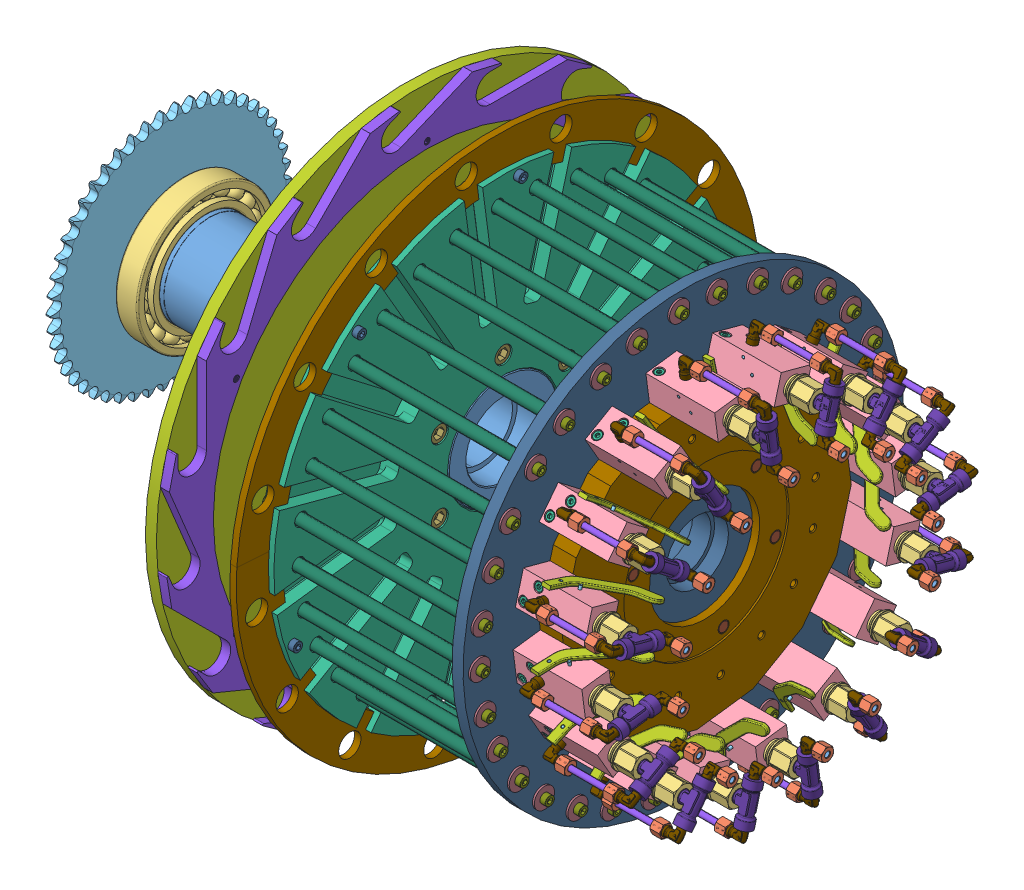
SolidWorks assembly assieme parte rotante, configuration Default. Lengths in mm. (continued)
Components (placement in the parent): (continued)
- AssiemeValvola-7: AssiemeValvola [Default] at (515.3257 -116.5064 518.4894) x (0 0.793353 -0.608761) z (0 -0.608761 -0.793353) size (90.26 138.63 38)
  - RaccordoT-1: RaccordoT [Default] at origin size (43 29.75 16.5)
  - Raccordo a L-1: Raccordo a L [Default] at (-30 0 0) x (0 -1 0) z (0 0 -1) size (28.34 25.51 14.01)
    - 1809_06_10_01-1: 1809_06_10_01 [Default] at origin size (22.49 23 10)
    - 1809_06_10_02-1: 1809_06_10_02 [Default] at origin size (6.5 8.5 8.5)
    - 1809_06_10_03-1: 1809_06_10_03 [Default] at origin size (11.02 15.01 14.01)
  - Raccordo a L-2: Raccordo a L [Default] at (30 0 0) x (0 1 0) z (0 0 -1) size (28.34 25.51 14.01)
    - 1809_06_10_01-1: 1809_06_10_01 [Default] at origin size (22.49 23 10)
    - 1809_06_10_02-1: 1809_06_10_02 [Default] at origin size (6.5 8.5 8.5)
    - 1809_06_10_03-1: 1809_06_10_03 [Default] at origin size (11.02 15.01 14.01)
  - TappoChiusura-1: TappoChiusura [Default] at (0 -32 0) x (0 -1 0) z (0 0 1) size (38.28 26.74 26.74)
  - CorpoValvola-1: CorpoValvola [Default] at (-15 -115.2824 0) size (30 75 34)
  - Raccordo a L-3: Raccordo a L [Default] at (-30 -88.2824 0) x (0 1 0) z (0 0 1) size (28.34 25.51 14.01)
    - 1809_06_10_01-1: 1809_06_10_01 [Default] at origin size (22.49 23 10)
    - 1809_06_10_02-1: 1809_06_10_02 [Default] at origin size (6.5 8.5 8.5)
    - 1809_06_10_03-1: 1809_06_10_03 [Default] at origin size (11.02 15.01 14.01)
  - Spina_3x38-1: Spina_3x38 [Default] at (0 -68.2824 -21) x (-1 0 0) z (0 0 1) size (3 3 38)
  - Spina_3x38-2: Spina_3x38 [Default] at (-10 -80.2824 -21) x (0.996193 0.087174 0) z (0 0 1) size (3 3 38)
  - M5 40mm-3: M5 40mm [ISO 4762 M5 x 40 - 40N] at (-14.6 -108.7824 9) size (45 8.5 8.5)
  - M5 40mm-2: M5 40mm [ISO 4762 M5 x 40 - 40N] at (-14.6 -96.7824 -9) size (45 8.5 8.5)
  - LevaValvola-1: LevaValvola [Default] at (-24.507 -86.571 -17) x (0.996193 0.087174 0) z (0 0 1) size (77.55 60.2 4)
  - Tubo-1: Tubo [Default] at (-30 -15.9665 0) x (1 0 0) z (0 -1 0) size (6 6 56.4)
- AssiemeValvola-8: AssiemeValvola [Default] at (515.3257 -66.6363 562.2243) x (0 0.5 -0.866025) z (0 -0.866025 -0.5) size (90.26 138.63 38)
  - RaccordoT-1: RaccordoT [Default] at origin size (43 29.75 16.5)
  - Raccordo a L-1: Raccordo a L [Default] at (-30 0 0) x (0 -1 0) z (0 0 -1) size (28.34 25.51 14.01)
    - 1809_06_10_01-1: 1809_06_10_01 [Default] at origin size (22.49 23 10)
    - 1809_06_10_02-1: 1809_06_10_02 [Default] at origin size (6.5 8.5 8.5)
    - 1809_06_10_03-1: 1809_06_10_03 [Default] at origin size (11.02 15.01 14.01)
  - Raccordo a L-2: Raccordo a L [Default] at (30 0 0) x (0 1 0) z (0 0 -1) size (28.34 25.51 14.01)
    - 1809_06_10_01-1: 1809_06_10_01 [Default] at origin size (22.49 23 10)
    - 1809_06_10_02-1: 1809_06_10_02 [Default] at origin size (6.5 8.5 8.5)
    - 1809_06_10_03-1: 1809_06_10_03 [Default] at origin size (11.02 15.01 14.01)
  - TappoChiusura-1: TappoChiusura [Default] at (0 -32 0) x (0 -1 0) z (0 0 1) size (38.28 26.74 26.74)
  - CorpoValvola-1: CorpoValvola [Default] at (-15 -115.2824 0) size (30 75 34)
  - Raccordo a L-3: Raccordo a L [Default] at (-30 -88.2824 0) x (0 1 0) z (0 0 1) size (28.34 25.51 14.01)
    - 1809_06_10_01-1: 1809_06_10_01 [Default] at origin size (22.49 23 10)
    - 1809_06_10_02-1: 1809_06_10_02 [Default] at origin size (6.5 8.5 8.5)
    - 1809_06_10_03-1: 1809_06_10_03 [Default] at origin size (11.02 15.01 14.01)
  - Spina_3x38-1: Spina_3x38 [Default] at (0 -68.2824 -21) x (-1 0 0) z (0 0 1) size (3 3 38)
  - Spina_3x38-2: Spina_3x38 [Default] at (-10 -80.2824 -21) x (0.996193 0.087174 0) z (0 0 1) size (3 3 38)
  - M5 40mm-3: M5 40mm [ISO 4762 M5 x 40 - 40N] at (-14.6 -108.7824 9) size (45 8.5 8.5)
  - M5 40mm-2: M5 40mm [ISO 4762 M5 x 40 - 40N] at (-14.6 -96.7824 -9) size (45 8.5 8.5)
  - LevaValvola-1: LevaValvola [Default] at (-24.507 -86.571 -17) x (0.996193 0.087174 0) z (0 0 1) size (77.55 60.2 4)
  - Tubo-1: Tubo [Default] at (-30 -15.9665 0) x (1 0 0) z (0 -1 0) size (6 6 56.4)
- AssiemeValvola-9: AssiemeValvola [Default] at (515.3257 -3.8258 583.5456) x (0 0.130526 -0.991445) z (0 -0.991445 -0.130526) size (90.26 138.63 38)
  - RaccordoT-1: RaccordoT [Default] at origin size (43 29.75 16.5)
  - Raccordo a L-1: Raccordo a L [Default] at (-30 0 0) x (0 -1 0) z (0 0 -1) size (28.34 25.51 14.01)
    - 1809_06_10_01-1: 1809_06_10_01 [Default] at origin size (22.49 23 10)
    - 1809_06_10_02-1: 1809_06_10_02 [Default] at origin size (6.5 8.5 8.5)
    - 1809_06_10_03-1: 1809_06_10_03 [Default] at origin size (11.02 15.01 14.01)
  - Raccordo a L-2: Raccordo a L [Default] at (30 0 0) x (0 1 0) z (0 0 -1) size (28.34 25.51 14.01)
    - 1809_06_10_01-1: 1809_06_10_01 [Default] at origin size (22.49 23 10)
    - 1809_06_10_02-1: 1809_06_10_02 [Default] at origin size (6.5 8.5 8.5)
    - 1809_06_10_03-1: 1809_06_10_03 [Default] at origin size (11.02 15.01 14.01)
  - TappoChiusura-1: TappoChiusura [Default] at (0 -32 0) x (0 -1 0) z (0 0 1) size (38.28 26.74 26.74)
  - CorpoValvola-1: CorpoValvola [Default] at (-15 -115.2824 0) size (30 75 34)
  - Raccordo a L-3: Raccordo a L [Default] at (-30 -88.2824 0) x (0 1 0) z (0 0 1) size (28.34 25.51 14.01)
    - 1809_06_10_01-1: 1809_06_10_01 [Default] at origin size (22.49 23 10)
    - 1809_06_10_02-1: 1809_06_10_02 [Default] at origin size (6.5 8.5 8.5)
    - 1809_06_10_03-1: 1809_06_10_03 [Default] at origin size (11.02 15.01 14.01)
  - Spina_3x38-1: Spina_3x38 [Default] at (0 -68.2824 -21) x (-1 0 0) z (0 0 1) size (3 3 38)
  - Spina_3x38-2: Spina_3x38 [Default] at (-10 -80.2824 -21) x (0.996193 0.087174 0) z (0 0 1) size (3 3 38)
  - M5 40mm-3: M5 40mm [ISO 4762 M5 x 40 - 40N] at (-14.6 -108.7824 9) size (45 8.5 8.5)
  - M5 40mm-2: M5 40mm [ISO 4762 M5 x 40 - 40N] at (-14.6 -96.7824 -9) size (45 8.5 8.5)
  - LevaValvola-1: LevaValvola [Default] at (-24.507 -86.571 -17) x (0.996193 0.087174 0) z (0 0 1) size (77.55 60.2 4)
  - Tubo-1: Tubo [Default] at (-30 -15.9665 0) x (1 0 0) z (0 -1 0) size (6 6 56.4)
- AssiemeValvola-10: AssiemeValvola [Default] at (515.3257 62.3629 579.2074) x (0 -0.258819 -0.965926) z (0 -0.965926 0.258819) size (90.26 138.63 38)
  - RaccordoT-1: RaccordoT [Default] at origin size (43 29.75 16.5)
  - Raccordo a L-1: Raccordo a L [Default] at (-30 0 0) x (0 -1 0) z (0 0 -1) size (28.34 25.51 14.01)
    - 1809_06_10_01-1: 1809_06_10_01 [Default] at origin size (22.49 23 10)
    - 1809_06_10_02-1: 1809_06_10_02 [Default] at origin size (6.5 8.5 8.5)
    - 1809_06_10_03-1: 1809_06_10_03 [Default] at origin size (11.02 15.01 14.01)
  - Raccordo a L-2: Raccordo a L [Default] at (30 0 0) x (0 1 0) z (0 0 -1) size (28.34 25.51 14.01)
    - 1809_06_10_01-1: 1809_06_10_01 [Default] at origin size (22.49 23 10)
    - 1809_06_10_02-1: 1809_06_10_02 [Default] at origin size (6.5 8.5 8.5)
    - 1809_06_10_03-1: 1809_06_10_03 [Default] at origin size (11.02 15.01 14.01)
  - TappoChiusura-1: TappoChiusura [Default] at (0 -32 0) x (0 -1 0) z (0 0 1) size (38.28 26.74 26.74)
  - CorpoValvola-1: CorpoValvola [Default] at (-15 -115.2824 0) size (30 75 34)
  - Raccordo a L-3: Raccordo a L [Default] at (-30 -88.2824 0) x (0 1 0) z (0 0 1) size (28.34 25.51 14.01)
    - 1809_06_10_01-1: 1809_06_10_01 [Default] at origin size (22.49 23 10)
    - 1809_06_10_02-1: 1809_06_10_02 [Default] at origin size (6.5 8.5 8.5)
    - 1809_06_10_03-1: 1809_06_10_03 [Default] at origin size (11.02 15.01 14.01)
  - Spina_3x38-1: Spina_3x38 [Default] at (0 -68.2824 -21) x (-1 0 0) z (0 0 1) size (3 3 38)
  - Spina_3x38-2: Spina_3x38 [Default] at (-10 -80.2824 -21) x (0.996193 0.087174 0) z (0 0 1) size (3 3 38)
  - M5 40mm-3: M5 40mm [ISO 4762 M5 x 40 - 40N] at (-14.6 -108.7824 9) size (45 8.5 8.5)
  - M5 40mm-2: M5 40mm [ISO 4762 M5 x 40 - 40N] at (-14.6 -96.7824 -9) size (45 8.5 8.5)
  - LevaValvola-1: LevaValvola [Default] at (-24.507 -86.571 -17) x (0.996193 0.087174 0) z (0 0 1) size (77.55 60.2 4)
  - Tubo-1: Tubo [Default] at (-30 -15.9665 0) x (1 0 0) z (0 -1 0) size (6 6 56.4)
- AssiemeValvola-11: AssiemeValvola [Default] at (515.3257 121.8531 549.8701) x (0 -0.608761 -0.793353) z (0 -0.793353 0.608761) size (90.26 138.63 38)
  - RaccordoT-1: RaccordoT [Default] at origin size (43 29.75 16.5)
  - Raccordo a L-1: Raccordo a L [Default] at (-30 0 0) x (0 -1 0) z (0 0 -1) size (28.34 25.51 14.01)
    - 1809_06_10_01-1: 1809_06_10_01 [Default] at origin size (22.49 23 10)
    - 1809_06_10_02-1: 1809_06_10_02 [Default] at origin size (6.5 8.5 8.5)
    - 1809_06_10_03-1: 1809_06_10_03 [Default] at origin size (11.02 15.01 14.01)
  - Raccordo a L-2: Raccordo a L [Default] at (30 0 0) x (0 1 0) z (0 0 -1) size (28.34 25.51 14.01)
    - 1809_06_10_01-1: 1809_06_10_01 [Default] at origin size (22.49 23 10)
    - 1809_06_10_02-1: 1809_06_10_02 [Default] at origin size (6.5 8.5 8.5)
    - 1809_06_10_03-1: 1809_06_10_03 [Default] at origin size (11.02 15.01 14.01)
  - TappoChiusura-1: TappoChiusura [Default] at (0 -32 0) x (0 -1 0) z (0 0 1) size (38.28 26.74 26.74)
  - CorpoValvola-1: CorpoValvola [Default] at (-15 -115.2824 0) size (30 75 34)
  - Raccordo a L-3: Raccordo a L [Default] at (-30 -88.2824 0) x (0 1 0) z (0 0 1) size (28.34 25.51 14.01)
    - 1809_06_10_01-1: 1809_06_10_01 [Default] at origin size (22.49 23 10)
    - 1809_06_10_02-1: 1809_06_10_02 [Default] at origin size (6.5 8.5 8.5)
    - 1809_06_10_03-1: 1809_06_10_03 [Default] at origin size (11.02 15.01 14.01)
  - Spina_3x38-1: Spina_3x38 [Default] at (0 -68.2824 -21) x (-1 0 0) z (0 0 1) size (3 3 38)
  - Spina_3x38-2: Spina_3x38 [Default] at (-10 -80.2824 -21) x (0.996193 0.087174 0) z (0 0 1) size (3 3 38)
  - M5 40mm-3: M5 40mm [ISO 4762 M5 x 40 - 40N] at (-14.6 -108.7824 9) size (45 8.5 8.5)
  - M5 40mm-2: M5 40mm [ISO 4762 M5 x 40 - 40N] at (-14.6 -96.7824 -9) size (45 8.5 8.5)
  - LevaValvola-1: LevaValvola [Default] at (-24.507 -86.571 -17) x (0.996193 0.087174 0) z (0 0 1) size (77.55 60.2 4)
  - Tubo-1: Tubo [Default] at (-30 -15.9665 0) x (1 0 0) z (0 -1 0) size (6 6 56.4)
- AssiemeValvola-12: AssiemeValvola [Default] at (515.3257 165.588 500) x (0 -0.866025 -0.5) z (0 -0.5 0.866025) size (90.26 138.63 38)
  - RaccordoT-1: RaccordoT [Default] at origin size (43 29.75 16.5)
  - Raccordo a L-1: Raccordo a L [Default] at (-30 0 0) x (0 -1 0) z (0 0 -1) size (28.34 25.51 14.01)
    - 1809_06_10_01-1: 1809_06_10_01 [Default] at origin size (22.49 23 10)
    - 1809_06_10_02-1: 1809_06_10_02 [Default] at origin size (6.5 8.5 8.5)
    - 1809_06_10_03-1: 1809_06_10_03 [Default] at origin size (11.02 15.01 14.01)
  - Raccordo a L-2: Raccordo a L [Default] at (30 0 0) x (0 1 0) z (0 0 -1) size (28.34 25.51 14.01)
    - 1809_06_10_01-1: 1809_06_10_01 [Default] at origin size (22.49 23 10)
    - 1809_06_10_02-1: 1809_06_10_02 [Default] at origin size (6.5 8.5 8.5)
    - 1809_06_10_03-1: 1809_06_10_03 [Default] at origin size (11.02 15.01 14.01)
  - TappoChiusura-1: TappoChiusura [Default] at (0 -32 0) x (0 -1 0) z (0 0 1) size (38.28 26.74 26.74)
  - CorpoValvola-1: CorpoValvola [Default] at (-15 -115.2824 0) size (30 75 34)
  - Raccordo a L-3: Raccordo a L [Default] at (-30 -88.2824 0) x (0 1 0) z (0 0 1) size (28.34 25.51 14.01)
    - 1809_06_10_01-1: 1809_06_10_01 [Default] at origin size (22.49 23 10)
    - 1809_06_10_02-1: 1809_06_10_02 [Default] at origin size (6.5 8.5 8.5)
    - 1809_06_10_03-1: 1809_06_10_03 [Default] at origin size (11.02 15.01 14.01)
  - Spina_3x38-1: Spina_3x38 [Default] at (0 -68.2824 -21) x (-1 0 0) z (0 0 1) size (3 3 38)
  - Spina_3x38-2: Spina_3x38 [Default] at (-10 -80.2824 -21) x (0.996193 0.087174 0) z (0 0 1) size (3 3 38)
  - M5 40mm-3: M5 40mm [ISO 4762 M5 x 40 - 40N] at (-14.6 -108.7824 9) size (45 8.5 8.5)
  - M5 40mm-2: M5 40mm [ISO 4762 M5 x 40 - 40N] at (-14.6 -96.7824 -9) size (45 8.5 8.5)
  - LevaValvola-1: LevaValvola [Default] at (-24.507 -86.571 -17) x (0.996193 0.087174 0) z (0 0 1) size (77.55 60.2 4)
  - Tubo-1: Tubo [Default] at (-30 -15.9665 0) x (1 0 0) z (0 -1 0) size (6 6 56.4)
- AssiemeValvola-13: AssiemeValvola [Default] at (515.3257 186.9093 437.1895) x (0 -0.991445 -0.130526) z (0 -0.130526 0.991445) size (90.26 138.63 38)
  - RaccordoT-1: RaccordoT [Default] at origin size (43 29.75 16.5)
  - Raccordo a L-1: Raccordo a L [Default] at (-30 0 0) x (0 -1 0) z (0 0 -1) size (28.34 25.51 14.01)
    - 1809_06_10_01-1: 1809_06_10_01 [Default] at origin size (22.49 23 10)
    - 1809_06_10_02-1: 1809_06_10_02 [Default] at origin size (6.5 8.5 8.5)
    - 1809_06_10_03-1: 1809_06_10_03 [Default] at origin size (11.02 15.01 14.01)
  - Raccordo a L-2: Raccordo a L [Default] at (30 0 0) x (0 1 0) z (0 0 -1) size (28.34 25.51 14.01)
    - 1809_06_10_01-1: 1809_06_10_01 [Default] at origin size (22.49 23 10)
    - 1809_06_10_02-1: 1809_06_10_02 [Default] at origin size (6.5 8.5 8.5)
    - 1809_06_10_03-1: 1809_06_10_03 [Default] at origin size (11.02 15.01 14.01)
  - TappoChiusura-1: TappoChiusura [Default] at (0 -32 0) x (0 -1 0) z (0 0 1) size (38.28 26.74 26.74)
  - CorpoValvola-1: CorpoValvola [Default] at (-15 -115.2824 0) size (30 75 34)
  - Raccordo a L-3: Raccordo a L [Default] at (-30 -88.2824 0) x (0 1 0) z (0 0 1) size (28.34 25.51 14.01)
    - 1809_06_10_01-1: 1809_06_10_01 [Default] at origin size (22.49 23 10)
    - 1809_06_10_02-1: 1809_06_10_02 [Default] at origin size (6.5 8.5 8.5)
    - 1809_06_10_03-1: 1809_06_10_03 [Default] at origin size (11.02 15.01 14.01)
  - Spina_3x38-1: Spina_3x38 [Default] at (0 -68.2824 -21) x (-1 0 0) z (0 0 1) size (3 3 38)
  - Spina_3x38-2: Spina_3x38 [Default] at (-10 -80.2824 -21) x (0.996193 0.087174 0) z (0 0 1) size (3 3 38)
  - M5 40mm-3: M5 40mm [ISO 4762 M5 x 40 - 40N] at (-14.6 -108.7824 9) size (45 8.5 8.5)
  - M5 40mm-2: M5 40mm [ISO 4762 M5 x 40 - 40N] at (-14.6 -96.7824 -9) size (45 8.5 8.5)
  - LevaValvola-1: LevaValvola [Default] at (-24.507 -86.571 -17) x (0.996193 0.087174 0) z (0 0 1) size (77.55 60.2 4)
  - Tubo-1: Tubo [Default] at (-30 -15.9665 0) x (1 0 0) z (0 -1 0) size (6 6 56.4)
- AssiemeValvola-14: AssiemeValvola [Default] at (515.3257 182.5711 371.0008) x (0 -0.965926 0.258819) z (0 0.258819 0.965926) size (90.26 138.63 38)
  - RaccordoT-1: RaccordoT [Default] at origin size (43 29.75 16.5)
  - Raccordo a L-1: Raccordo a L [Default] at (-30 0 0) x (0 -1 0) z (0 0 -1) size (28.34 25.51 14.01)
    - 1809_06_10_01-1: 1809_06_10_01 [Default] at origin size (22.49 23 10)
    - 1809_06_10_02-1: 1809_06_10_02 [Default] at origin size (6.5 8.5 8.5)
    - 1809_06_10_03-1: 1809_06_10_03 [Default] at origin size (11.02 15.01 14.01)
  - Raccordo a L-2: Raccordo a L [Default] at (30 0 0) x (0 1 0) z (0 0 -1) size (28.34 25.51 14.01)
    - 1809_06_10_01-1: 1809_06_10_01 [Default] at origin size (22.49 23 10)
    - 1809_06_10_02-1: 1809_06_10_02 [Default] at origin size (6.5 8.5 8.5)
    - 1809_06_10_03-1: 1809_06_10_03 [Default] at origin size (11.02 15.01 14.01)
  - TappoChiusura-1: TappoChiusura [Default] at (0 -32 0) x (0 -1 0) z (0 0 1) size (38.28 26.74 26.74)
  - CorpoValvola-1: CorpoValvola [Default] at (-15 -115.2824 0) size (30 75 34)
  - Raccordo a L-3: Raccordo a L [Default] at (-30 -88.2824 0) x (0 1 0) z (0 0 1) size (28.34 25.51 14.01)
    - 1809_06_10_01-1: 1809_06_10_01 [Default] at origin size (22.49 23 10)
    - 1809_06_10_02-1: 1809_06_10_02 [Default] at origin size (6.5 8.5 8.5)
    - 1809_06_10_03-1: 1809_06_10_03 [Default] at origin size (11.02 15.01 14.01)
  - Spina_3x38-1: Spina_3x38 [Default] at (0 -68.2824 -21) x (-1 0 0) z (0 0 1) size (3 3 38)
  - Spina_3x38-2: Spina_3x38 [Default] at (-10 -80.2824 -21) x (0.996193 0.087174 0) z (0 0 1) size (3 3 38)
  - M5 40mm-3: M5 40mm [ISO 4762 M5 x 40 - 40N] at (-14.6 -108.7824 9) size (45 8.5 8.5)
  - M5 40mm-2: M5 40mm [ISO 4762 M5 x 40 - 40N] at (-14.6 -96.7824 -9) size (45 8.5 8.5)
  - LevaValvola-1: LevaValvola [Default] at (-24.507 -86.571 -17) x (0.996193 0.087174 0) z (0 0 1) size (77.55 60.2 4)
  - Tubo-1: Tubo [Default] at (-30 -15.9665 0) x (1 0 0) z (0 -1 0) size (6 6 56.4)
- AssiemeValvola-15: AssiemeValvola [Default] at (515.3257 153.2338 311.5106) x (0 -0.793353 0.608761) z (0 0.608761 0.793353) size (90.26 138.63 38)
  - RaccordoT-1: RaccordoT [Default] at origin size (43 29.75 16.5)
  - Raccordo a L-1: Raccordo a L [Default] at (-30 0 0) x (0 -1 0) z (0 0 -1) size (28.34 25.51 14.01)
    - 1809_06_10_01-1: 1809_06_10_01 [Default] at origin size (22.49 23 10)
    - 1809_06_10_02-1: 1809_06_10_02 [Default] at origin size (6.5 8.5 8.5)
    - 1809_06_10_03-1: 1809_06_10_03 [Default] at origin size (11.02 15.01 14.01)
  - Raccordo a L-2: Raccordo a L [Default] at (30 0 0) x (0 1 0) z (0 0 -1) size (28.34 25.51 14.01)
    - 1809_06_10_01-1: 1809_06_10_01 [Default] at origin size (22.49 23 10)
    - 1809_06_10_02-1: 1809_06_10_02 [Default] at origin size (6.5 8.5 8.5)
    - 1809_06_10_03-1: 1809_06_10_03 [Default] at origin size (11.02 15.01 14.01)
  - TappoChiusura-1: TappoChiusura [Default] at (0 -32 0) x (0 -1 0) z (0 0 1) size (38.28 26.74 26.74)
  - CorpoValvola-1: CorpoValvola [Default] at (-15 -115.2824 0) size (30 75 34)
  - Raccordo a L-3: Raccordo a L [Default] at (-30 -88.2824 0) x (0 1 0) z (0 0 1) size (28.34 25.51 14.01)
    - 1809_06_10_01-1: 1809_06_10_01 [Default] at origin size (22.49 23 10)
    - 1809_06_10_02-1: 1809_06_10_02 [Default] at origin size (6.5 8.5 8.5)
    - 1809_06_10_03-1: 1809_06_10_03 [Default] at origin size (11.02 15.01 14.01)
  - Spina_3x38-1: Spina_3x38 [Default] at (0 -68.2824 -21) x (-1 0 0) z (0 0 1) size (3 3 38)
  - Spina_3x38-2: Spina_3x38 [Default] at (-10 -80.2824 -21) x (0.996193 0.087174 0) z (0 0 1) size (3 3 38)
  - M5 40mm-3: M5 40mm [ISO 4762 M5 x 40 - 40N] at (-14.6 -108.7824 9) size (45 8.5 8.5)
  - M5 40mm-2: M5 40mm [ISO 4762 M5 x 40 - 40N] at (-14.6 -96.7824 -9) size (45 8.5 8.5)
  - LevaValvola-1: LevaValvola [Default] at (-24.507 -86.571 -17) x (0.996193 0.087174 0) z (0 0 1) size (77.55 60.2 4)
  - Tubo-1: Tubo [Default] at (-30 -15.9665 0) x (1 0 0) z (0 -1 0) size (6 6 56.4)
- AssiemeValvola-16: AssiemeValvola [Default] at (515.3257 103.3637 267.7757) x (0 -0.5 0.866025) z (0 0.866025 0.5) size (90.26 138.63 38)
  - RaccordoT-1: RaccordoT [Default] at origin size (43 29.75 16.5)
  - Raccordo a L-1: Raccordo a L [Default] at (-30 0 0) x (0 -1 0) z (0 0 -1) size (28.34 25.51 14.01)
    - 1809_06_10_01-1: 1809_06_10_01 [Default] at origin size (22.49 23 10)
    - 1809_06_10_02-1: 1809_06_10_02 [Default] at origin size (6.5 8.5 8.5)
    - 1809_06_10_03-1: 1809_06_10_03 [Default] at origin size (11.02 15.01 14.01)
  - Raccordo a L-2: Raccordo a L [Default] at (30 0 0) x (0 1 0) z (0 0 -1) size (28.34 25.51 14.01)
    - 1809_06_10_01-1: 1809_06_10_01 [Default] at origin size (22.49 23 10)
    - 1809_06_10_02-1: 1809_06_10_02 [Default] at origin size (6.5 8.5 8.5)
    - 1809_06_10_03-1: 1809_06_10_03 [Default] at origin size (11.02 15.01 14.01)
  - TappoChiusura-1: TappoChiusura [Default] at (0 -32 0) x (0 -1 0) z (0 0 1) size (38.28 26.74 26.74)
  - CorpoValvola-1: CorpoValvola [Default] at (-15 -115.2824 0) size (30 75 34)
  - Raccordo a L-3: Raccordo a L [Default] at (-30 -88.2824 0) x (0 1 0) z (0 0 1) size (28.34 25.51 14.01)
    - 1809_06_10_01-1: 1809_06_10_01 [Default] at origin size (22.49 23 10)
    - 1809_06_10_02-1: 1809_06_10_02 [Default] at origin size (6.5 8.5 8.5)
    - 1809_06_10_03-1: 1809_06_10_03 [Default] at origin size (11.02 15.01 14.01)
  - Spina_3x38-1: Spina_3x38 [Default] at (0 -68.2824 -21) x (-1 0 0) z (0 0 1) size (3 3 38)
  - Spina_3x38-2: Spina_3x38 [Default] at (-10 -80.2824 -21) x (0.996193 0.087174 0) z (0 0 1) size (3 3 38)
  - M5 40mm-3: M5 40mm [ISO 4762 M5 x 40 - 40N] at (-14.6 -108.7824 9) size (45 8.5 8.5)
  - M5 40mm-2: M5 40mm [ISO 4762 M5 x 40 - 40N] at (-14.6 -96.7824 -9) size (45 8.5 8.5)
  - LevaValvola-1: LevaValvola [Default] at (-24.507 -86.571 -17) x (0.996193 0.087174 0) z (0 0 1) size (77.55 60.2 4)
  - Tubo-1: Tubo [Default] at (-30 -15.9665 0) x (1 0 0) z (0 -1 0) size (6 6 56.4)
- Disco alimentazione guarnizione fi24.4-1: Disco alimentazione guarnizione fi24.4 [Default] at (198.0433 18.3637 415) x (0 0.065403 0.997859) z (-1 0 0) size (570 285 7.35)
- Disco alimentazione guarnizione fi24.4-2: Disco alimentazione guarnizione fi24.4 [Default] at (198.0433 18.3637 415) x (0 -0.065403 -0.997859) z (-1 0 0) size (570 285 7.35)
- m6 12mm-1: m6 12mm [ISO 4762 M6 x 12 - 12N] at (210.0433 200.6849 574.8914) x (-1 0 0) z (0 0.793353 -0.608761) size (18 10 10)
- m6 12mm-7: m6 12mm [ISO 4762 M6 x 12 - 12N] at (210.0433 260.3445 399.1397) x (-1 0 0) z (0 0.793353 -0.608761) size (18 10 10)
- m6 12mm-8: m6 12mm [ISO 4762 M6 x 12 - 12N] at (210.0433 96.3128 185.3694) x (-1 0 0) z (0 0.793353 -0.608761) size (18 10 10)
- m6 12mm-9: m6 12mm [ISO 4762 M6 x 12 - 12N] at (210.0433 -59.5854 644.6306) x (-1 0 0) z (0 -0.793353 -0.608761) size (18 10 10)
- m6 12mm-10: m6 12mm [ISO 4762 M6 x 12 - 12N] at (210.0433 -223.6171 430.8603) x (-1 0 0) z (0 -0.793353 -0.608761) size (18 10 10)
- m6 12mm-11: m6 12mm [ISO 4762 M6 x 12 - 12N] at (210.0433 -163.9575 255.1086) x (-1 0 0) z (0 0.793353 -0.608761) size (18 10 10)
Mates (geometry in assembly coordinates):
- Concentrico1: concentric anti-aligned: circle of albero rotazione piatti-1; circle of seger 100mm-1
- Coincidente1: coincident anti-aligned: plane of albero rotazione piatti-1 through (-143.4567 18.3637 415) normal (-1 0 0); plane of seger 100mm-2 through (-143.4567 18.3637 415) normal (1 0 0)
- Coincidente2: coincident aligned: plane of albero rotazione piatti-1 through (60.413 18.3637 415) normal (0 1 0); plane of seger 100mm-2 through (-146.4567 18.3637 415) normal (0 1 0)
- Concentrico21: concentric aligned: cylinder of albero rotazione piatti-1 through (60.413 18.3637 415) axis (1 0 0) radius 50; cylinder of SKF - 6020 - 20,DE,NC,20_68-1 through (-152.0942 18.3637 415) axis (1 0 0) radius 50
- Coincidente3: coincident anti-aligned: plane of seger 100mm-2 through (-143.4567 18.3637 415) normal (1 0 0); plane of SKF - 6020 - 20,DE,NC,20_68-1 through (-143.4567 -33.4256 439.9823) normal (-1 0 0)
- Concentrico3: concentric aligned: cylinder of albero rotazione piatti-1 through (60.413 18.3637 415) axis (1 0 0) radius 47.5; cylinder of calettatore d95-1 through (-188.8867 18.3637 415) axis (1 0 0) radius 47.5
- Coincidente7: coincident aligned: plane of albero rotazione piatti-1 through (60.413 18.3637 415) normal (0 1 0); plane of calettatore d95-1 through (-173.8867 18.3637 415) normal (0 1 0)
- Concentrico5: concentric aligned: cylinder of albero rotazione piatti-1 through (60.413 18.3637 415) axis (1 0 0) radius 49.75; cylinder of SKF - 6020 - 20,DE,NC,20_68-2 through (41.4058 18.3637 415) axis (1 0 0) radius 50
- Coincidente8: coincident anti-aligned: plane of albero rotazione piatti-1 through (74.0433 18.3637 415) normal (-1 0 0); plane of SKF - 6020 - 20,DE,NC,20_68-2 through (74.0433 -28.0673 437.2803) normal (1 0 0)
- Concentrico6: concentric aligned: cylinder of albero rotazione piatti-1 through (60.413 18.3637 415) axis (1 0 0) radius 60; cylinder of Disco supporto montaggio e Colonne-1 through (5.3377 18.3637 415) axis (1 0 0) radius 60
- Concentrico7: concentric aligned: cylinder of albero rotazione piatti-1 through (101.3656 98.3637 415) axis (1 0 0) radius 6.25; cylinder of Disco supporto montaggio e Colonne-1 through (204.0433 98.3637 415) axis (1 0 0) radius 9.25
- Coincidente9: coincident anti-aligned: plane of albero rotazione piatti-1 through (175.0433 18.3637 415) normal (1 0 0); plane of Disco supporto montaggio e Colonne-1 through (175.0433 18.3637 415) normal (-1 0 0)
- Concentrico8: concentric anti-aligned: cylinder of albero rotazione piatti-1 through (60.413 18.3637 415) axis (1 0 0) radius 60; cylinder of piatto rotante porta tappi-1 through (111.0433 18.3637 415) axis (-1 0 0) radius 60
- Concentrico9: concentric aligned: circle of albero rotazione piatti-1; circle of piatto rotante porta tappi-1
- Coincidente10: coincident anti-aligned: plane of albero rotazione piatti-1 through (119.0433 18.3637 415) normal (-1 0 0); plane of piatto rotante porta tappi-1 through (119.0433 18.3637 415) normal (1 0 0)
- Concentrico10: concentric aligned: cylinder of piatto rotante porta tappi-1 through (119.0433 18.3637 415) axis (-1 0 0) radius 233; cylinder of disco trasportatore tappi 31-1 through (121.0433 18.3637 415) axis (-1 0 0) radius 233
- Concentrico323: concentric aligned: cylinder of piatto rotante porta tappi-1 through (98.5243 -101.6363 622.8461) axis (1 0 0) radius 3.25; circle of disco trasportatore tappi 31-1
- Coincidente13: coincident anti-aligned: plane of piatto rotante porta tappi-1 through (111.0433 18.3637 415) normal (1 0 0); plane of disco trasportatore tappi 31-1 through (111.0433 18.3637 415) normal (-1 0 0)
- Concentrico11: concentric anti-aligned: cylinder of albero rotazione piatti-1 through (60.413 18.3637 415) axis (1 0 0) radius 40; cylinder of disco trascinato porta distributore vuoto-1 through (400.0433 18.3637 415) axis (-1 0 0) radius 30
- Concentrico12: concentric anti-aligned: cylinder of Disco supporto montaggio e Colonne-1 through (204.0433 -202.0247 450.2415) axis (1 0 0) radius 6; cylinder of disco trascinato porta distributore vuoto-1 through (417.0139 -202.0247 450.2415) axis (-1 0 0) radius 6
- Coincidente14: coincident anti-aligned: plane of Distributore Rotante-1 through (400.0433 18.3637 415) normal (-1 0 0); plane of disco trascinato porta distributore vuoto-1 through (400.0433 18.3637 415) normal (1 0 0)
- Concentrico13: concentric anti-aligned: circle of Distributore Rotante-1; circle of disco trascinato porta distributore vuoto-1
- Concentrico14: concentric anti-aligned: cylinder of Distributore Rotante-1 through (230.3377 18.3637 415) axis (1 0 0) radius 60; cylinder of disco trascinato porta distributore vuoto-1 through (415.0433 18.3637 415) axis (-1 0 0) radius 67.5
- Concentrico15: concentric anti-aligned: cylinder of disco trascinato porta distributore vuoto-1 through (388.0433 -58.9104 394.2945) axis (1 0 0) radius 6.25; cylinder of m12 35mm-1 through (344.2933 -58.9104 394.2945) axis (-1 0 0) radius 6
- Coincidente15: coincident anti-aligned: plane of disco trascinato porta distributore vuoto-1 through (388.0433 18.3637 415) normal (-1 0 0); plane of m12 35mm-1 through (388.0433 -51.1161 398.7945) normal (1 0 0)
- Parallelo1: parallel anti-aligned: plane of m12 35mm-1 through (382.0433 -53.8529 397.2144) normal (0 -1 0)
- Concentrico16: concentric aligned: cylinder of Disco supporto montaggio e Colonne-1 through (204.0433 -21.6363 345.718) axis (1 0 0) radius 9.25; cylinder of m12 90mm-3 through (234.7933 -21.6363 345.718) axis (1 0 0) radius 6
- Coincidente17: coincident anti-aligned: plane of Disco supporto montaggio e Colonne-1 through (191.0433 -27.049 342.593) normal (1 0 0); plane of m12 90mm-3 through (191.0433 -29.4305 341.218) normal (-1 0 0)
- Parallelo2: parallel aligned: plane of m12 35mm-1 through (382.0433 -53.8529 397.2144) normal (0 -1 0); plane of m12 90mm-3 through (197.0433 -16.5788 348.6379) normal (0 -1 0)
- Concentrico171: concentric anti-aligned: cylinder of piatto rotante porta tappi-1 through (98.5243 -101.6363 207.1539) axis (1 0 0) radius 3.25; cylinder of rondella M6-1 through (64.1183 -101.6363 207.1539) axis (-1 0 0) radius 3.3
- Coincidente191: coincident anti-aligned: plane of piatto rotante porta tappi-1 through (99.0433 18.3637 415) normal (-1 0 0); plane of rondella M6-1 through (99.0433 -101.6363 210.4539) normal (1 0 0)
- Parallelo3: parallel anti-aligned: plane of rondella M6-1 through (99.0433 -101.6363 207.1539) normal (0 -1 0)
- Concentrico181: concentric aligned: cylinder of rondella M6-1 through (64.1183 -101.6363 207.1539) axis (-1 0 0) radius 3.3; cylinder of M6 20mm-1 through (59.2933 -101.6363 207.1539) axis (-1 0 0) radius 5
- Coincidente211: coincident anti-aligned: plane of rondella M6-1 through (97.0433 -101.6363 218.1539) normal (-1 0 0); plane of M6 20mm-1 through (97.0433 -97.3062 204.6539) normal (1 0 0)
- Parallelo4: parallel aligned: plane of m12 35mm-1 through (382.0433 -53.8529 397.2144) normal (0 -0.5 -0.866025); plane of M6 20mm-1 through (94.0433 -101.6363 210.0892) normal (0 -0.5 -0.866025)
- Concentrico19: concentric anti-aligned: cylinder of Disco supporto montaggio e Colonne-1 through (204.0433 70.1437 197.9013) axis (1 0 0) radius 6; cylinder of asta scorrimento carello-1 through (400.0433 70.1437 197.9013) axis (-1 0 0) radius 6
- Concentrico201: concentric aligned: cylinder of asta scorrimento carello-1 through (175.0433 70.1437 197.9013) axis (-1 0 0) radius 3.2; cylinder of rondella M6-7 through (140.1183 70.1437 197.9013) axis (-1 0 0) radius 3.3
- Coincidente231: coincident anti-aligned: plane of asta scorrimento carello-1 through (175.0433 70.1437 197.9013) normal (-1 0 0); plane of rondella M6-7 through (175.0433 70.1437 201.2013) normal (1 0 0)
- Concentrico211: concentric aligned: cylinder of rondella M6-7 through (140.1183 70.1437 197.9013) axis (-1 0 0) radius 3.3; cylinder of M6 16mm-1 through (135.2933 70.1437 197.9013) axis (-1 0 0) radius 5
- Coincidente241: coincident anti-aligned: plane of rondella M6-7 through (173.0433 70.1437 208.9013) normal (-1 0 0); plane of M6 16mm-1 through (173.0433 75.1437 197.9013) normal (1 0 0)
- Parallelo5: parallel aligned: plane of asta scorrimento carello-1 through (287.5433 70.1437 197.9013) normal (0 0 -1); plane of M6 16mm-1 through (170.0433 68.6761 200.4433) normal (0 0 -1)
- Parallelo9: parallel anti-aligned: plane of rondella M6-7 through (175.0433 70.1437 197.9013) normal (0 0 1); plane of M6 16mm-1 through (170.0433 68.6761 200.4433) normal (0 0 -1)
- Coincidente30: coincident anti-aligned: plane of Disco supporto montaggio e Colonne-1 through (175.0433 18.3637 415) normal (-1 0 0); plane of rondella M6-7 through (175.0433 70.1437 201.2013) normal (1 0 0)
- Coincidente31: coincident anti-aligned: plane of disco trascinato porta distributore vuoto-1 through (400.0433 18.3637 415) normal (1 0 0); plane of rondella M6-26 through (400.0433 70.1437 201.2013) normal (-1 0 0)
- Coincidente32: coincident anti-aligned: plane of Distributore Rotante-1 through (400.0433 8.0276 257.3017) normal (0 0.130526 -0.991445); plane of AssiemeValvola-1/CorpoValvola-1 through (400.0433 55.4498 263.545) normal (0 -0.130526 0.991445)
- Coincidente33: coincident anti-aligned: plane of disco trascinato porta distributore vuoto-1 through (400.0433 18.3637 415) normal (1 0 0); plane of AssiemeValvola-1/CorpoValvola-1 through (400.0433 59.3656 233.8016) normal (-1 0 0)
- Concentrico22: concentric anti-aligned: cylinder of Distributore Rotante-1 through (412.5433 32.9826 303.9582) axis (0 0.130526 -0.991445) radius 3; cylinder of AssiemeValvola-1/CorpoValvola-1 through (412.5433 38.5953 261.326) axis (0 -0.130526 0.991445) radius 3
- Concentrico23: concentric anti-aligned: cylinder of Disco supporto montaggio e Colonne-1 through (198.0433 18.3637 415) axis (-1 0 0) radius 235; cylinder of Disco alimentazione guarnizione fi24.4-2 through (191.0433 18.3637 415) axis (1 0 0) radius 235
- Concentrico24: concentric anti-aligned: cylinder of Disco supporto montaggio e Colonne-1 through (198.0433 18.3637 415) axis (-1 0 0) radius 235; cylinder of Disco alimentazione guarnizione fi24.4-1 through (191.0433 18.3637 415) axis (1 0 0) radius 235
- Coincidente34: coincident anti-aligned: plane of Disco alimentazione guarnizione fi24.4-1 through (191.0433 33.7334 649.4968) normal (0 -0.997859 0.065403); plane of Disco alimentazione guarnizione fi24.4-2 through (191.0433 37.0036 699.3898) normal (0 0.997859 -0.065403)
- Coincidente35: coincident aligned: plane of Disco alimentazione guarnizione fi24.4-1 through (198.0433 18.3637 415) normal (1 0 0); plane of Disco alimentazione guarnizione fi24.4-2 through (198.0433 18.3637 415) normal (1 0 0)
- Concentrico25: concentric anti-aligned: cylinder of Disco supporto montaggio e Colonne-1 through (188.8509 -59.5854 644.6306) axis (1 0 0) radius 3.25; circle of Disco alimentazione guarnizione fi24.4-2
- Coincidente36: coincident anti-aligned: plane of Disco supporto montaggio e Colonne-1 through (198.0433 18.3637 415) normal (-1 0 0); plane of Disco alimentazione guarnizione fi24.4-2 through (198.0433 18.3637 415) normal (1 0 0)
- Concentrico26: concentric anti-aligned: cylinder of Disco supporto montaggio e Colonne-1 through (188.8509 200.6849 574.8914) axis (1 0 0) radius 3.25; cylinder of M6 16mm-65 through (198.0564 200.6849 574.8914) axis (-1 0 0) radius 3
- Concentrico271: concentric anti-aligned: cone of Disco supporto montaggio e Colonne-1 through (203.0433 200.6849 574.8914) axis (-1 0 0); cylinder of m6 12mm-1 through (241.7933 200.6849 574.8914) axis (1 0 0) radius 5
- Coincidente381: coincident anti-aligned: plane of Disco supporto montaggio e Colonne-1 through (204.0433 18.3637 415) normal (1 0 0); plane of m6 12mm-1 through (204.0433 203.7287 578.8581) normal (-1 0 0)
- Concentrico281: concentric anti-aligned: cylinder of Disco supporto montaggio e Colonne-1 through (203.0433 260.3445 399.1397) axis (-1 0 0) radius 785.3982; cylinder of m6 12mm-7 through (241.7933 260.3445 399.1397) axis (1 0 0) radius 5
- Coincidente401: coincident anti-aligned: plane of Disco supporto montaggio e Colonne-1 through (204.0433 18.3637 415) normal (1 0 0); plane of m6 12mm-7 through (204.0433 263.3883 403.1065) normal (-1 0 0)
- Parallelo11: parallel aligned: plane of m6 12mm-1 through (207.0433 198.898 572.5627) normal (0 0.92388 0.382683); plane of m6 12mm-7 through (207.0433 258.5576 396.8111) normal (0 0.92388 0.382683)
- Concentrico291: concentric anti-aligned: cylinder of Disco supporto montaggio e Colonne-1 through (203.0433 96.3128 185.3694) axis (-1 0 0) radius 785.3982; cylinder of m6 12mm-8 through (241.7933 96.3128 185.3694) axis (1 0 0) radius 5
- Coincidente421: coincident anti-aligned: plane of Disco supporto montaggio e Colonne-1 through (204.0433 18.3637 415) normal (1 0 0); plane of m6 12mm-8 through (204.0433 99.3566 189.3362) normal (-1 0 0)
- Coincidente44: coincident aligned: plane of m6 12mm-7 through (207.0433 259.2212 401.8516) normal (0 0.793353 -0.608761); plane of m6 12mm-8 through (207.0433 95.1895 188.0813) normal (0 0.793353 -0.608761)
- Concentrico301: concentric anti-aligned: cylinder of Disco supporto montaggio e Colonne-1 through (203.0433 -59.5854 644.6306) axis (-1 0 0) radius 785.3982; cylinder of m6 12mm-9 through (241.7933 -59.5854 644.6306) axis (1 0 0) radius 5
- Coincidente451: coincident anti-aligned: plane of Disco supporto montaggio e Colonne-1 through (204.0433 18.3637 415) normal (1 0 0); plane of m6 12mm-9 through (204.0433 -56.5416 640.6638) normal (-1 0 0)
- Concentrico311: concentric anti-aligned: cylinder of Disco supporto montaggio e Colonne-1 through (203.0433 -223.6171 430.8603) axis (-1 0 0) radius 785.3982; cylinder of m6 12mm-10 through (241.7933 -223.6171 430.8603) axis (1 0 0) radius 5
- Coincidente461: coincident anti-aligned: plane of Disco supporto montaggio e Colonne-1 through (204.0433 18.3637 415) normal (1 0 0); plane of m6 12mm-10 through (204.0433 -220.5733 426.8935) normal (-1 0 0)
- Concentrico321: concentric anti-aligned: cylinder of Disco supporto montaggio e Colonne-1 through (203.0433 -163.9575 255.1086) axis (-1 0 0) radius 785.3982; cylinder of m6 12mm-11 through (241.7933 -163.9575 255.1086) axis (1 0 0) radius 5
- Coincidente471: coincident anti-aligned: plane of Disco supporto montaggio e Colonne-1 through (204.0433 18.3637 415) normal (1 0 0); plane of m6 12mm-11 through (204.0433 -160.9136 259.0754) normal (-1 0 0)
- Parallelo13: parallel aligned: plane of m6 12mm-9 through (207.0433 -62.4955 644.2474) normal (0 0.92388 -0.382683); plane of m6 12mm-10 through (207.0433 -226.5272 430.4771) normal (0 0.92388 -0.382683)
- Parallelo14: parallel aligned: plane of Disco supporto montaggio e Colonne-1 through (191.0433 26.2972 408.9124) normal (0 -0.793353 0.608761); plane of m6 12mm-11 through (207.0433 -162.8342 252.3968) normal (0 -0.793353 0.608761)
- Parallelo15: parallel aligned: plane of Disco supporto montaggio e Colonne-1 through (191.0433 19.669 405.0856) normal (0 -0.130526 0.991445); plane of m6 12mm-10 through (207.0433 -221.8302 428.5316) normal (0 -0.130526 0.991445)
- Concentrico322: concentric anti-aligned: cylinder of albero rotazione piatti-1 through (60.413 18.3637 415) axis (1 0 0) radius 47.5; cylinder of Chain wheel ISO - 50Z 10A-1-1 through (-139.8862 18.3637 415) axis (-1 0 0) radius 47.5
- Coincidente472: coincident anti-aligned: plane of albero rotazione piatti-1 through (-155.9567 18.3637 415) normal (-1 0 0); plane of Chain wheel ISO - 50Z 10A-1-1 through (-155.9567 18.3637 415) normal (1 0 0)
- Parallelo16: parallel aligned: plane of Chain wheel ISO - 50Z 10A-1-1 through (-164.8867 18.3637 415) normal (0 1 0)
- Parallelo17: parallel aligned: plane of calettatore d95-1 through (-173.8867 18.3637 415) normal (0 1 0)
- Coincidente473: coincident anti-aligned: plane of calettatore d95-1 through (-159.8867 84.9137 415) normal (1 0 0); plane of Chain wheel ISO - 50Z 10A-1-1 through (-159.8867 18.3637 415) normal (-1 0 0)
